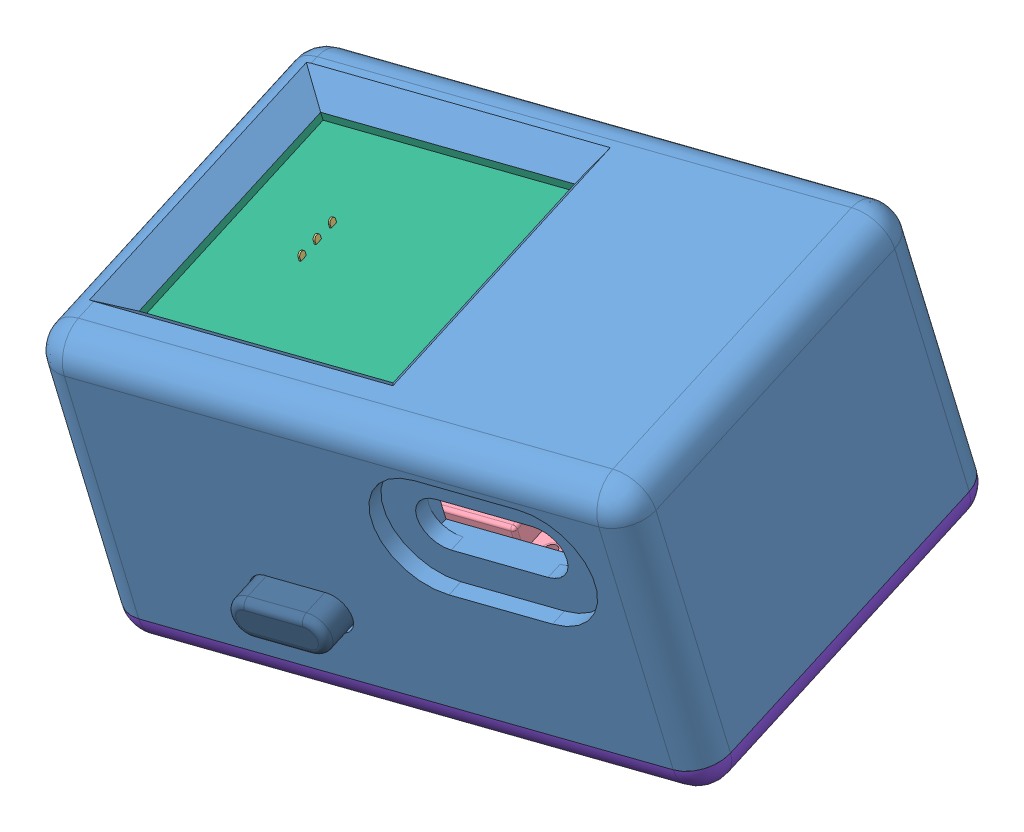
SolidWorks assembly 装配结果, configuration 默认. Lengths in mm.
Overall size (41.47 28.59 32.35).
10 component instances, 10 part files, 27 mates.
Components (placement in the parent):
- 底壳-1: 底壳 [默认] at (-70.1082 58.5981 -8.73) x (0.979335 0.14583 -0.14013) z (-0.166967 0.191999 -0.967088) size (36 17.3 24)
- 滚轮-1: 滚轮 [默认] at (-103.708 42.4217 -31.5865) x (0.979335 0.14583 -0.14013) z (0.166967 -0.191999 0.967088) size (14.01 4.03 14.04)
- 3D_电源板_2025-01-22-1: 3D_电源板_2025-01-22 [默认] at (-133.8097 50.7162 -21.3514) x (-0.166967 0.191999 -0.967088) z (0.114125 -0.9705 -0.21238) size (18.99 24.09 5.8)
- 3D_主控板_2025-01-22-2: 3D_主控板_2025-01-22 [默认] at (-148.3029 45.1649 -38.1444) x (0.166967 -0.191999 0.967088) z (0.114125 -0.9705 -0.21238) size (19.69 23.99 7.92)
- 电池-1: 电池 [默认] at (-115.864 39.1299 -25.8123) x (0.166967 -0.191999 0.967088) z (-0.979335 -0.14583 0.14013) size (22 5 11)
- 屏幕-1: 屏幕 [默认] at (-134.9311 49.8659 -18.0686) x (-0.166967 0.191999 -0.967088) z (0.979335 0.14583 -0.14013) size (17.6 1.56 21.8)
- 排线-1: 排线 [默认] at (-110.3953 50.8456 -26.0534) x (0.114125 -0.9705 -0.21238) z (-0.979335 -0.14583 0.14013) size (8 8 3)
- 盖子-1: 盖子 [默认] at (-47.4773 25.1414 74.8585) x (0.166967 -0.191999 0.967088) z (0.114125 -0.9705 -0.21238) size (24 36 6)
- 金属方轴-1: 金属方轴 [默认] at (-132.8831 42.2762 -28.8291) x (0.979335 0.14583 -0.14013) z (0.166967 -0.191999 0.967088) size (0.8 5.4 0.8)
- 按钮-1: 按钮 [默认] at (-130.7052 37.085 -10.5531) x (0.979335 0.14583 -0.14013) z (0.166967 -0.191999 0.967088) size (11.5 4 4)
Mates (geometry in assembly coordinates):
- 重合4: coincident anti-aligned: plane of 滚轮-1 through (-132.2711 41.0247 -28.78) normal (-0.114125 0.9705 0.21238); plane of 3D_主控板_2025-01-22-2 through (-134.477 41.0307 -29.993) normal (0.114125 -0.9705 -0.21238)
- 重合24: coincident: line of 底壳-1 through (-127.0403 54.4404 -27.3869) axis (-0.979335 -0.14583 0.14013); plane of 屏幕-1 through (-141.879 51.7371 -25.3617) normal (0.166967 -0.191999 0.967088)
- 重合26: coincident: line of 底壳-1 through (-141.936 52.2224 -25.2555) axis (0.166967 -0.191999 0.967088); plane of 屏幕-1 through (-139.3394 48.8168 -10.6523) normal (0.979335 0.14583 -0.14013)
- 重合30: coincident anti-aligned: plane of 底壳-1 through (-108.5959 51.8022 -12.4825) normal (-0.979335 -0.14583 0.14013); plane of 排线-1 through (-110.3953 50.8456 -26.0534) normal (0.979335 0.14583 -0.14013)
- 重合37: coincident anti-aligned: plane of 底壳-1 through (-69.937 57.1424 -9.0485) normal (0.114125 -0.9705 -0.21238); plane of 屏幕-1 through (-135.1092 51.3799 -17.7373) normal (-0.114125 0.9705 0.21238)
- 重合40: coincident anti-aligned: plane of 3D_电源板_2025-01-22-1 through (-114.8734 51.9797 -25.4247) normal (-0.979335 -0.14583 0.14013); plane of 3D_主控板_2025-01-22-2 through (-114.0413 44.8542 -27.0243) normal (0.979335 0.14583 -0.14013)
- 重合41: coincident anti-aligned: plane of 3D_电源板_2025-01-22-1 through (-115.4466 52.0027 -25.8381) normal (0.166967 -0.191999 0.967088); plane of 3D_主控板_2025-01-22-2 through (-114.5022 46.5146 -27.0908) normal (-0.166967 0.191999 -0.967088)
- 重合42: coincident anti-aligned: plane of 3D_主控板_2025-01-22-2 through (-110.8625 44.4156 -14.6014) normal (0.979335 0.14583 -0.14013); plane of 排线-1 through (-113.3333 50.4081 -25.6331) normal (-0.979335 -0.14583 0.14013)
- 重合43: coincident anti-aligned: plane of 底壳-1 through (-143.274 50.9756 -27.3401) normal (0.166967 -0.191999 0.967088); plane of 3D_主控板_2025-01-22-2 through (-114.0333 48.0618 -32.967) normal (-0.166967 0.191999 -0.967088)
- 重合50: coincident anti-aligned: plane of 底壳-1 through (-69.7658 55.6866 -9.3671) normal (0.114125 -0.9705 -0.21238); plane of 排线-1 through (-113.0366 53.0927 -20.7659) normal (-0.114125 0.9705 0.21238)
- 重合58: coincident: plane of 底壳-1 through (-143.9346 37.1898 -32.031) normal (-0.166967 0.191999 -0.967088); line of 盖子-1 through (-141.9759 37.4815 -32.3113) axis (0.979335 0.14583 -0.14013)
- 重合59: coincident anti-aligned: plane of 底壳-1 through (-68.1338 41.8085 -12.4041) normal (0.114125 -0.9705 -0.21238); plane of 盖子-1 through (-47.4773 25.1414 74.8585) normal (-0.114125 0.9705 0.21238)
- 重合60: coincident: plane of 底壳-1 through (-143.9346 37.1898 -32.031) normal (-0.979335 -0.14583 0.14013); line of 盖子-1 through (-140.2613 32.9658 -10.7551) axis (-0.166967 0.191999 -0.967088)
- 重合61: coincident anti-aligned: plane of 滚轮-1 through (-103.708 42.4217 -31.5865) normal (-0.114125 0.9705 0.21238); plane of 金属方轴-1 through (-132.3188 38.4599 -28.857) normal (0.114125 -0.9705 -0.21238)
- 重合62: coincident anti-aligned: plane of 滚轮-1 through (-132.4558 38.6173 -29.65) normal (0.979335 0.14583 -0.14013); plane of 金属方轴-1 through (-132.9351 43.7006 -27.7101) normal (-0.979335 -0.14583 0.14013)
- 重合63: coincident anti-aligned: plane of 滚轮-1 through (-132.3188 38.4599 -28.857) normal (-0.166967 0.191999 -0.967088); plane of 金属方轴-1 through (-132.7495 42.1226 -28.0555) normal (0.166967 -0.191999 0.967088)
- 重合64: coincident anti-aligned: plane of 3D_主控板_2025-01-22-2 through (-132.2206 41.7069 -29.0565) normal (0.166967 -0.191999 0.967088); plane of 金属方轴-1 through (-132.8831 42.2762 -28.8291) normal (-0.166967 0.191999 -0.967088)
- 重合65: coincident anti-aligned: plane of 3D_主控板_2025-01-22-2 through (-132.7061 41.505 -28.3948) normal (0.979335 0.14583 -0.14013); plane of 金属方轴-1 through (-132.9351 43.7006 -27.7101) normal (-0.979335 -0.14583 0.14013)
- 距离1: distance = 8.3 mm anti-aligned: plane of 3D_主控板_2025-01-22-2 through (-124.081 43.5189 -22.3157) normal (0.114125 -0.9705 -0.21238); plane of 3D_电源板_2025-01-22-1 through (-125.247 51.5469 -20.5461) normal (-0.114125 0.9705 0.21238)
- 重合72: coincident anti-aligned: plane of 底壳-1 through (-114.3724 54.6287 -28.5026) normal (0.166967 -0.191999 0.967088); plane of 排线-1 through (-114.3724 54.6287 -28.5026) normal (-0.166967 0.191999 -0.967088)
- 重合78: coincident anti-aligned: plane of 底壳-1 through (-124.7515 44.7669 -32.8047) normal (0.166967 -0.191999 0.967088); plane of 电池-1 through (-113.9789 46.371 -34.3461) normal (-0.166967 0.191999 -0.967088)
- 重合79: coincident anti-aligned: plane of 底壳-1 through (-68.7045 46.661 -11.3422) normal (0.114125 -0.9705 -0.21238); plane of 电池-1 through (-116.4347 43.9824 -24.7504) normal (-0.114125 0.9705 0.21238)
- 重合80: coincident anti-aligned: plane of 底壳-1 through (-124.5846 44.5749 -31.8376) normal (0.979335 0.14583 -0.14013); plane of 电池-1 through (-124.7515 44.7669 -32.8047) normal (-0.979335 -0.14583 0.14013)
- 重合81: coincident anti-aligned: plane of 3D_电源板_2025-01-22-1 through (-125.247 51.5469 -20.5461) normal (-0.114125 0.9705 0.21238); plane of 屏幕-1 through (-134.9311 49.8659 -18.0686) normal (0.114125 -0.9705 -0.21238)
- 重合82: coincident anti-aligned: plane of 底壳-1 through (-124.0415 39.3117 -11.2616) normal (-0.166967 0.191999 -0.967088); plane of 按钮-1 through (-130.7052 37.085 -10.5531) normal (0.166967 -0.191999 0.967088)
- 平行4: parallel anti-aligned: plane of 底壳-1 through (-125.9861 40.0394 -9.7463) normal (0.114125 -0.9705 -0.21238); plane of 按钮-1 through (-129.2597 39.0691 -7.3067) normal (-0.114125 0.9705 0.21238)
- 距离2: distance = 0 mm: cylinder of 按钮-1 through (-129.1228 37.9045 -7.5616) axis (-0.166967 0.191999 -0.967088) radius 1.2; cylinder of 底壳-1 through (-129.4565 38.2883 -9.4948) axis (-0.166967 0.191999 -0.967088) radius 1.2643
